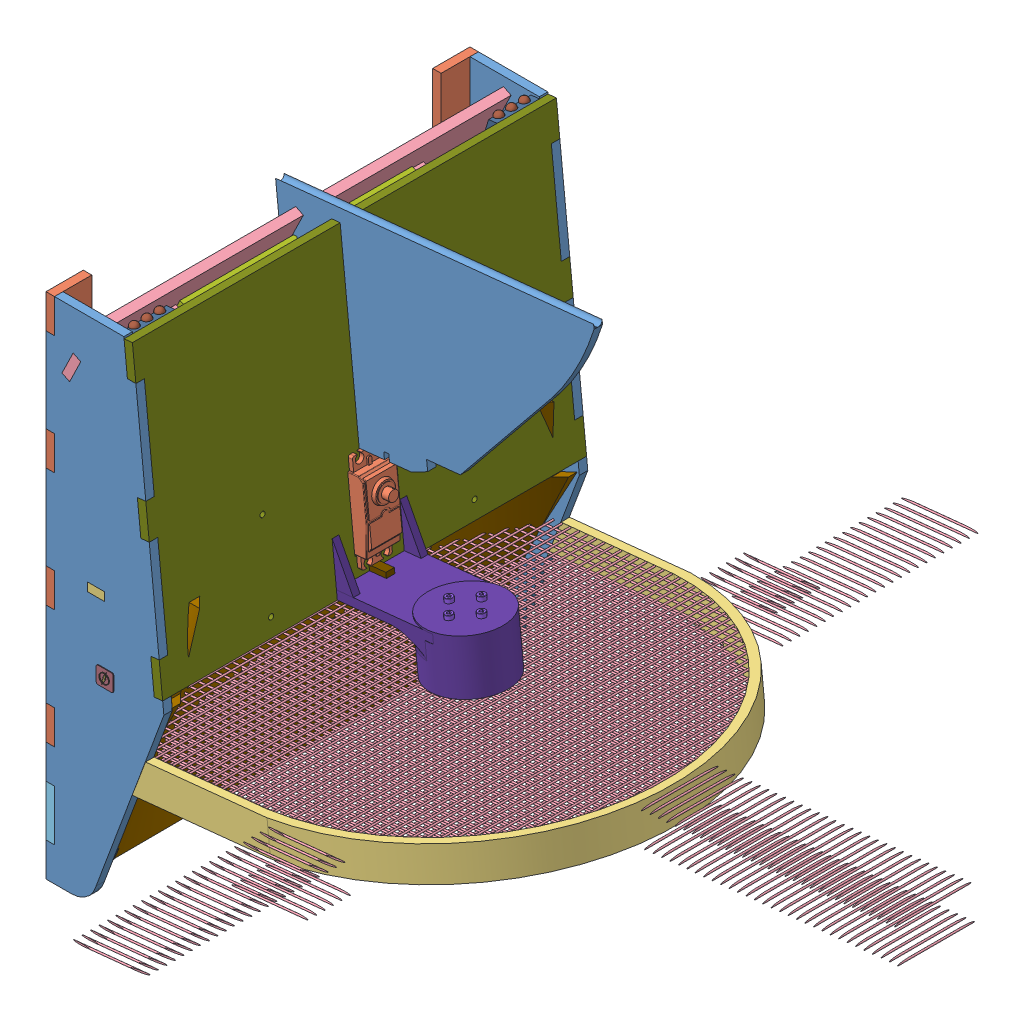
SolidWorks assembly AssStructSimu, configuration Défaut. Lengths in mm. (continued)
Components (placement in the parent): (continued)
- AssCarte-1: AssCarte [Défaut] at (38.0121 147.1029 290.772) x (-0.101852 0.9948 0) z (0.9948 0.101852 0) size (66.52 130.57 98.72) (hidden) (continued)
  - carte_onduleur_v3-1: carte_onduleur_v3 [Défaut] at (-131.8199 12.0892 20.7912) size (66.52 130.57 82.34) (continued)
    - CON_IO1-1: CON_IO1 [Défaut] at (-11.3 12.1 0.803) x (0 -1 0) z (0 0 1) size (13 30 57.5) (continued)
      - Open CASCADE STEP translator 6.8 1.3.1-1: Open CASCADE STEP translator 6.8 1.3.1 [Défaut] at origin size (13 30 57.5) (continued)
        - Body_1_2-1: Body_1_2 [Défaut] at (-3 -15 8) x (0 -1 0) z (-1 0 0) size (30 57.5 13) (continued)
          - 74-1: 74 [Défaut] at (-4.9 41.8 0.803) x (0 -1 0) z (0 0 1) size (6 4.9 1.75) (continued)
            - =_[0_1_1_56]-1: =_[0_1_1_56] [Défaut] at origin size (6 4.9 1.75) (continued)
              - 72-1: 72 [Défaut] at origin size (6 4.9 1.75)
                - =_[0_1_1_2]-1: =_[0_1_1_2] [Défaut] at origin size (3.9 4.9 1.57)
                - =_[0_1_1_3]-1: =_[0_1_1_3] [Défaut] at origin size (6 4.22 1)
                  - =_[0_1_1_60]-1: =_[0_1_1_60] [Défaut] at origin size (1.05 0.41 1)
                  - =_[0_1_1_61]-1: =_[0_1_1_61] [Défaut] at origin size (1.05 0.41 1)
                  - =_[0_1_1_62]-1: =_[0_1_1_62] [Défaut] at origin size (1.05 0.41 1)
                  - =_[0_1_1_63]-1: =_[0_1_1_63] [Défaut] at origin size (1.05 0.41 1)
                  - =_[0_1_1_64]-1: =_[0_1_1_64] [Défaut] at origin size (1.05 0.41 1)
                  - =_[0_1_1_65]-1: =_[0_1_1_65] [Défaut] at origin size (1.05 0.41 1)
                  - =_[0_1_1_66]-1: =_[0_1_1_66] [Défaut] at origin size (1.05 0.41 1)
                  - =_[0_1_1_67]-1: =_[0_1_1_67] [Défaut] at origin size (1.05 0.41 1)
          - 76-1: 76 [Défaut] at (-8.5 40.5664 0.803) x (0 1 0) z (0 0 1) size (2.34 1.04 0.5)
            - =_[0_1_1_42]-1: =_[0_1_1_42] [Défaut] at origin size (2.34 1.04 0.5)
              - 43-1: 43 [Défaut] at origin size (2.29 1.04 0.43)
              - 44-1: 44 [Défaut] at (0.3048 0 0) x (-1 0 0) z (0 0 1) size (0.51 1.02 0.5)
              - 45-1: 45 [Défaut] at origin size (0.51 1.02 0.5)
          - 78-1: 78 [Défaut] at (-5.9 46.4 0.803) x (-1 0 0) z (0 0 1) size (2.34 1.04 0.5)
            - =_[0_1_1_42]-1: =_[0_1_1_42] [Défaut] at origin size (2.34 1.04 0.5)
              - 43-1: 43 [Défaut] at origin size (2.29 1.04 0.43)
              - 44-1: 44 [Défaut] at (0.3048 0 0) x (-1 0 0) z (0 0 1) size (0.51 1.02 0.5)
              - 45-1: 45 [Défaut] at origin size (0.51 1.02 0.5)
          - 80-1: 80 [Défaut] at (-7 48.1 0.803) size (2.34 1.04 0.5)
            - =_[0_1_1_42]-1: =_[0_1_1_42] [Défaut] at origin size (2.34 1.04 0.5)
              - 43-1: 43 [Défaut] at origin size (2.29 1.04 0.43)
              - 44-1: 44 [Défaut] at (0.3048 0 0) x (-1 0 0) z (0 0 1) size (0.51 1.02 0.5)
              - 45-1: 45 [Défaut] at origin size (0.51 1.02 0.5)
          - 82-1: 82 [Défaut] at (-6 37.1 0.803) size (2.34 1.04 0.5)
            - =_[0_1_1_42]-1: =_[0_1_1_42] [Défaut] at origin size (2.34 1.04 0.5)
              - 43-1: 43 [Défaut] at origin size (2.29 1.04 0.43)
              - 44-1: 44 [Défaut] at (0.3048 0 0) x (-1 0 0) z (0 0 1) size (0.51 1.02 0.5)
              - 45-1: 45 [Défaut] at origin size (0.51 1.02 0.5)
    - CON_IO2-1: CON_IO2 [Défaut] at (-11.3 -2.7 0.803) x (0 -1 0) z (0 0 1) size (13 30 57.5)
      - Open CASCADE STEP translator 6.8 1.4.1-1: Open CASCADE STEP translator 6.8 1.4.1 [Défaut] at origin size (13 30 57.5)
        - Body_1_2-1: Body_1_2 [Défaut] at (-3 -15 8) x (0 -1 0) z (-1 0 0) size (30 57.5 13)
          - 1-1: 1 [Défaut] at origin size (30 50 1.61)
          - 10-1: 10 [Défaut] at (-14.395 31.0465 0.803) x (-1 0 0) z (0 0 1) size (5.59 6.35 1.11)
            - =_[0_1_1_4]-1: =_[0_1_1_4] [Défaut] at origin size (5.59 6.35 1.11)
              - 11-1: 11 [Défaut] at (2 3.3 0) x (-1 0 0) z (0 0 1) size (5.59 6.35 1.11)
                - =_[0_1_1_3]_2-1: =_[0_1_1_3]_2 [Défaut] at origin size (0.44 0.55 0.36)
                - =_[0_1_1_4]_2-1: =_[0_1_1_4]_2 [Défaut] at origin size (5.59 4.15 0.36)
                - =_[0_1_1_5]_2-1: =_[0_1_1_5]_2 [Défaut] at origin size (5.35 6.1 1.1)
                - =_[0_1_1_6]-1: =_[0_1_1_6] [Défaut] at origin size (0.44 0.55 0.36)
                - =_[0_1_1_7]-1: =_[0_1_1_7] [Défaut] at origin size (0.44 0.55 0.36)
                - =_[0_1_1_8]-1: =_[0_1_1_8] [Défaut] at origin size (0.44 0.55 0.36)
          - 13-1: 13 [Défaut] at (-12.62 16.6 -0.803) x (-1 0 0) z (0 0 -1) size (5.59 6.35 1.11)
            - =_[0_1_1_13]-1: =_[0_1_1_13] [Défaut] at origin size (5.59 6.35 1.11)
              - 11-1: 11 [Défaut] at (2 3.3 0) x (-1 0 0) z (0 0 1) size (5.59 6.35 1.11)
                - =_[0_1_1_3]_2-1: =_[0_1_1_3]_2 [Défaut] at origin size (0.44 0.55 0.36)
                - =_[0_1_1_4]_2-1: =_[0_1_1_4]_2 [Défaut] at origin size (5.59 4.15 0.36)
                - =_[0_1_1_5]_2-1: =_[0_1_1_5]_2 [Défaut] at origin size (5.35 6.1 1.1)
                - =_[0_1_1_6]-1: =_[0_1_1_6] [Défaut] at origin size (0.44 0.55 0.36)
                - =_[0_1_1_7]-1: =_[0_1_1_7] [Défaut] at origin size (0.44 0.55 0.36)
                - =_[0_1_1_8]-1: =_[0_1_1_8] [Défaut] at origin size (0.44 0.55 0.36)
          - 16-1: 16 [Défaut] at (-4.2 24.2 0.803) x (-1 0 0) z (0 0 1) size (12.8 0.5 13)
            - =_[0_1_1_15]-1: =_[0_1_1_15] [Défaut] at origin size (12.8 0.5 13)
              - 17-1: 17 [Défaut] at (2.7 0 0) x (1 0 0) z (0 -1 0) size (12.8 13 0.5)
          - 19-1: 19 [Défaut] at (-4.1 6.8 0.803) x (-1 0 0) z (0 0 1) size (12.8 0.5 13)
            - =_[0_1_1_18]-1: =_[0_1_1_18] [Défaut] at origin size (12.8 0.5 13)
              - 17-1: 17 [Défaut] at (2.7 0 0) x (1 0 0) z (0 -1 0) size (12.8 13 0.5)
          - 24-1: 24 [Défaut] at (-8.1 16.5 -0.803) x (0 1 0) z (0 0 -1) size (7.75 5.13 1.17)
            - =_[0_1_1_20]-1: =_[0_1_1_20] [Défaut] at origin size (7.75 5.13 1.17)
              - 20-1: 20 [Défaut] at origin size (7.59 5.13 1.07)
              - 21-1: 21 [Défaut] at (-14.478 0 0) x (-1 0 0) z (0 0 1) size (0.76 5.08 1.17)
              - 22-1: 22 [Défaut] at origin size (0.76 5.08 1.17)
          - 35-1: 35 [Défaut] at (-25.3 25.5 0.803) x (0 -1 0) z (0 0 1) size (6.05 5.2 1.7)
            - =_[0_1_1_25]-1: =_[0_1_1_25] [Défaut] at origin size (6.05 5.2 1.7)
              - 25-1: 25 [Défaut] at origin size (4.3 5.2 1.53)
              - 26-1: 26 [Défaut] at origin size (0.88 0.51 1.06)
              - 27-1: 27 [Défaut] at origin size (0.88 0.51 1.06)
              - 28-1: 28 [Défaut] at origin size (0.88 0.51 1.06)
              - 29-1: 29 [Défaut] at origin size (0.88 0.51 1.06)
              - 30-1: 30 [Défaut] at (11.6 -5.08 0) x (-1 0 0) z (0 0 1) size (0.87 0.51 1.06)
              - 31-1: 31 [Défaut] at (11.6 -2.54 0) x (-1 0 0) z (0 0 1) size (0.87 0.51 1.06)
              - 32-1: 32 [Défaut] at (11.6 0 0) x (-1 0 0) z (0 0 1) size (0.87 0.51 1.06)
              - 33-1: 33 [Défaut] at (11.6 2.54 0) x (-1 0 0) z (0 0 1) size (0.87 0.51 1.06)
          - 40-1: 40 [Défaut] at (-27.6 27.2 0.803) size (2.34 1.04 0.5)
            - =_[0_1_1_36]-1: =_[0_1_1_36] [Défaut] at origin size (2.34 1.04 0.5)
              - 36-1: 36 [Défaut] at origin size (2.29 1.04 0.43)
              - 37-1: 37 [Défaut] at (0.3048 0 0) x (-1 0 0) z (0 0 1) size (0.51 1.02 0.5)
              - 38-1: 38 [Défaut] at origin size (0.51 1.02 0.5)
          - 42-1: 42 [Défaut] at (-22.1 21.6 0.803) x (0 1 0) z (0 0 1) size (2.34 1.04 0.5)
            - =_[0_1_1_36]-1: =_[0_1_1_36] [Défaut] at origin size (2.34 1.04 0.5)
              - 36-1: 36 [Défaut] at origin size (2.29 1.04 0.43)
              - 37-1: 37 [Défaut] at (0.3048 0 0) x (-1 0 0) z (0 0 1) size (0.51 1.02 0.5)
              - 38-1: 38 [Défaut] at origin size (0.51 1.02 0.5)
          - 47-1: 47 [Défaut] at (-14.7664 14.5 -0.803) x (-1 0 0) z (0 0 -1) size (2.34 1.04 0.5)
            - =_[0_1_1_42]-1: =_[0_1_1_42] [Défaut] at origin size (2.34 1.04 0.5)
              - 43-1: 43 [Défaut] at origin size (2.29 1.04 0.43)
              - 44-1: 44 [Défaut] at (0.3048 0 0) x (-1 0 0) z (0 0 1) size (0.51 1.02 0.5)
              - 45-1: 45 [Défaut] at origin size (0.51 1.02 0.5)
          - 57-1: 57 [Défaut] at (-15.3 2.7 -0.803) x (0 -1 0) z (0 0 -1) size (10.36 15.24 6.14)
            - =_[0_1_1_47]-1: =_[0_1_1_47] [Défaut] at origin size (10.36 15.24 6.14)
              - 55-1: 55 [Défaut] at (1.8 -1.2 3) x (1 0 0) z (0 1 0) size (10.36 6.14 15.24)
                - 54-1: 54 [Défaut] at origin size (10.36 6.14 7.62)
                  - 52-1: 52 [Défaut] at origin size (10.36 6.14 2.54)
                    - 48-1: 48 [Défaut] at origin size (8.4 2.54 2.54)
                    - 49-1: 49 [Défaut] at (-0.0461 1.2682 1.27) x (0 0 -1) z (0.999998 -0.002105 0) size (1.95 5.07 7.58)
                  - 52-2: 52 [Défaut] at (0 0 -2.54) size (10.36 6.14 2.54)
                    - 48-1: 48 [Défaut] at origin size (8.4 2.54 2.54)
                    - 49-1: 49 [Défaut] at (-0.0461 1.2682 1.27) x (0 0 -1) z (0.999998 -0.002105 0) size (1.95 5.07 7.58)
                  - 52-3: 52 [Défaut] at (0 0 -5.08) size (10.36 6.14 2.54)
                    - 48-1: 48 [Défaut] at origin size (8.4 2.54 2.54)
                    - 49-1: 49 [Défaut] at (-0.0461 1.2682 1.27) x (0 0 -1) z (0.999998 -0.002105 0) size (1.95 5.07 7.58)
                - 54-2: 54 [Défaut] at (0 0 -7.62) size (10.36 6.14 7.62)
                  - 52-1: 52 [Défaut] at origin size (10.36 6.14 2.54)
                    - 48-1: 48 [Défaut] at origin size (8.4 2.54 2.54)
                    - 49-1: 49 [Défaut] at (-0.0461 1.2682 1.27) x (0 0 -1) z (0.999998 -0.002105 0) size (1.95 5.07 7.58)
                  - 52-2: 52 [Défaut] at (0 0 -2.54) size (10.36 6.14 2.54)
                    - 48-1: 48 [Défaut] at origin size (8.4 2.54 2.54)
                    - 49-1: 49 [Défaut] at (-0.0461 1.2682 1.27) x (0 0 -1) z (0.999998 -0.002105 0) size (1.95 5.07 7.58)
                  - 52-3: 52 [Défaut] at (0 0 -5.08) size (10.36 6.14 2.54)
                    - 48-1: 48 [Défaut] at origin size (8.4 2.54 2.54)
                    - 49-1: 49 [Défaut] at (-0.0461 1.2682 1.27) x (0 0 -1) z (0.999998 -0.002105 0) size (1.95 5.07 7.58)
          - 59-1: 59 [Défaut] at (-26.5 31 0.803) x (0 -1 0) z (0 0 1) size (2.34 1.04 0.5)
            - =_[0_1_1_42]-1: =_[0_1_1_42] [Défaut] at origin size (2.34 1.04 0.5)
              - 43-1: 43 [Défaut] at origin size (2.29 1.04 0.43)
              - 44-1: 44 [Défaut] at (0.3048 0 0) x (-1 0 0) z (0 0 1) size (0.51 1.02 0.5)
              - 45-1: 45 [Défaut] at origin size (0.51 1.02 0.5)
          - 61-1: 61 [Défaut] at (-21.6 17.8 0.803) x (-1 0 0) z (0 0 1) size (2.34 1.04 0.5)
            - =_[0_1_1_42]-1: =_[0_1_1_42] [Défaut] at origin size (2.34 1.04 0.5)
              - 43-1: 43 [Défaut] at origin size (2.29 1.04 0.43)
              - 44-1: 44 [Défaut] at (0.3048 0 0) x (-1 0 0) z (0 0 1) size (0.51 1.02 0.5)
              - 45-1: 45 [Défaut] at origin size (0.51 1.02 0.5)
          - 74-1: 74 [Défaut] at (-4.9 41.8 0.803) x (0 -1 0) z (0 0 1) size (6 4.9 1.75)
            - =_[0_1_1_56]-1: =_[0_1_1_56] [Défaut] at origin size (6 4.9 1.75)
              - 72-1: 72 [Défaut] at origin size (6 4.9 1.75)
                - =_[0_1_1_2]-1: =_[0_1_1_2] [Défaut] at origin size (3.9 4.9 1.57)
                - =_[0_1_1_3]-1: =_[0_1_1_3] [Défaut] at origin size (6 4.22 1)
                  - =_[0_1_1_60]-1: =_[0_1_1_60] [Défaut] at origin size (1.05 0.41 1)
                  - =_[0_1_1_61]-1: =_[0_1_1_61] [Défaut] at origin size (1.05 0.41 1)
                  - =_[0_1_1_62]-1: =_[0_1_1_62] [Défaut] at origin size (1.05 0.41 1)
                  - =_[0_1_1_63]-1: =_[0_1_1_63] [Défaut] at origin size (1.05 0.41 1)
                  - =_[0_1_1_64]-1: =_[0_1_1_64] [Défaut] at origin size (1.05 0.41 1)
                  - =_[0_1_1_65]-1: =_[0_1_1_65] [Défaut] at origin size (1.05 0.41 1)
                  - =_[0_1_1_66]-1: =_[0_1_1_66] [Défaut] at origin size (1.05 0.41 1)
                  - =_[0_1_1_67]-1: =_[0_1_1_67] [Défaut] at origin size (1.05 0.41 1)
          - 76-1: 76 [Défaut] at (-8.5 40.5664 0.803) x (0 1 0) z (0 0 1) size (2.34 1.04 0.5)
            - =_[0_1_1_42]-1: =_[0_1_1_42] [Défaut] at origin size (2.34 1.04 0.5)
              - 43-1: 43 [Défaut] at origin size (2.29 1.04 0.43)
              - 44-1: 44 [Défaut] at (0.3048 0 0) x (-1 0 0) z (0 0 1) size (0.51 1.02 0.5)
              - 45-1: 45 [Défaut] at origin size (0.51 1.02 0.5)
          - 78-1: 78 [Défaut] at (-5.9 46.4 0.803) x (-1 0 0) z (0 0 1) size (2.34 1.04 0.5)
            - =_[0_1_1_42]-1: =_[0_1_1_42] [Défaut] at origin size (2.34 1.04 0.5)
              - 43-1: 43 [Défaut] at origin size (2.29 1.04 0.43)
              - 44-1: 44 [Défaut] at (0.3048 0 0) x (-1 0 0) z (0 0 1) size (0.51 1.02 0.5)
              - 45-1: 45 [Défaut] at origin size (0.51 1.02 0.5)
          - 80-1: 80 [Défaut] at (-7 48.1 0.803) size (2.34 1.04 0.5)
            - =_[0_1_1_42]-1: =_[0_1_1_42] [Défaut] at origin size (2.34 1.04 0.5)
              - 43-1: 43 [Défaut] at origin size (2.29 1.04 0.43)
              - 44-1: 44 [Défaut] at (0.3048 0 0) x (-1 0 0) z (0 0 1) size (0.51 1.02 0.5)
              - 45-1: 45 [Défaut] at origin size (0.51 1.02 0.5)
          - 82-1: 82 [Défaut] at (-6 37.1 0.803) size (2.34 1.04 0.5)
            - =_[0_1_1_42]-1: =_[0_1_1_42] [Défaut] at origin size (2.34 1.04 0.5)
              - 43-1: 43 [Défaut] at origin size (2.29 1.04 0.43)
              - 44-1: 44 [Défaut] at (0.3048 0 0) x (-1 0 0) z (0 0 1) size (0.51 1.02 0.5)
              - 45-1: 45 [Défaut] at origin size (0.51 1.02 0.5)
    - CON_IO3-1: CON_IO3 [Défaut] at (-11.3 -17.7 0.803) x (0 -1 0) z (0 0 1) size (13 30 57.5)
      - Open CASCADE STEP translator 6.8 1.5.1-1: Open CASCADE STEP translator 6.8 1.5.1 [Défaut] at origin size (13 30 57.5)
        - Body_1_2-1: Body_1_2 [Défaut] at (-3 -15 8) x (0 -1 0) z (-1 0 0) size (30 57.5 13)
          - 1-1: 1 [Défaut] at origin size (30 50 1.61)
          - 10-1: 10 [Défaut] at (-14.395 31.0465 0.803) x (-1 0 0) z (0 0 1) size (5.59 6.35 1.11)
            - =_[0_1_1_4]-1: =_[0_1_1_4] [Défaut] at origin size (5.59 6.35 1.11)
              - 11-1: 11 [Défaut] at (2 3.3 0) x (-1 0 0) z (0 0 1) size (5.59 6.35 1.11)
                - =_[0_1_1_3]_2-1: =_[0_1_1_3]_2 [Défaut] at origin size (0.44 0.55 0.36)
                - =_[0_1_1_4]_2-1: =_[0_1_1_4]_2 [Défaut] at origin size (5.59 4.15 0.36)
                - =_[0_1_1_5]_2-1: =_[0_1_1_5]_2 [Défaut] at origin size (5.35 6.1 1.1)
                - =_[0_1_1_6]-1: =_[0_1_1_6] [Défaut] at origin size (0.44 0.55 0.36)
                - =_[0_1_1_7]-1: =_[0_1_1_7] [Défaut] at origin size (0.44 0.55 0.36)
                - =_[0_1_1_8]-1: =_[0_1_1_8] [Défaut] at origin size (0.44 0.55 0.36)
          - 13-1: 13 [Défaut] at (-12.62 16.6 -0.803) x (-1 0 0) z (0 0 -1) size (5.59 6.35 1.11)
            - =_[0_1_1_13]-1: =_[0_1_1_13] [Défaut] at origin size (5.59 6.35 1.11)
              - 11-1: 11 [Défaut] at (2 3.3 0) x (-1 0 0) z (0 0 1) size (5.59 6.35 1.11)
                - =_[0_1_1_3]_2-1: =_[0_1_1_3]_2 [Défaut] at origin size (0.44 0.55 0.36)
                - =_[0_1_1_4]_2-1: =_[0_1_1_4]_2 [Défaut] at origin size (5.59 4.15 0.36)
                - =_[0_1_1_5]_2-1: =_[0_1_1_5]_2 [Défaut] at origin size (5.35 6.1 1.1)
                - =_[0_1_1_6]-1: =_[0_1_1_6] [Défaut] at origin size (0.44 0.55 0.36)
                - =_[0_1_1_7]-1: =_[0_1_1_7] [Défaut] at origin size (0.44 0.55 0.36)
                - =_[0_1_1_8]-1: =_[0_1_1_8] [Défaut] at origin size (0.44 0.55 0.36)
          - 16-1: 16 [Défaut] at (-4.2 24.2 0.803) x (-1 0 0) z (0 0 1) size (12.8 0.5 13)
            - =_[0_1_1_15]-1: =_[0_1_1_15] [Défaut] at origin size (12.8 0.5 13)
              - 17-1: 17 [Défaut] at (2.7 0 0) x (1 0 0) z (0 -1 0) size (12.8 13 0.5)
          - 19-1: 19 [Défaut] at (-4.1 6.8 0.803) x (-1 0 0) z (0 0 1) size (12.8 0.5 13)
            - =_[0_1_1_18]-1: =_[0_1_1_18] [Défaut] at origin size (12.8 0.5 13)
              - 17-1: 17 [Défaut] at (2.7 0 0) x (1 0 0) z (0 -1 0) size (12.8 13 0.5)
          - 24-1: 24 [Défaut] at (-8.1 16.5 -0.803) x (0 1 0) z (0 0 -1) size (7.75 5.13 1.17)
            - =_[0_1_1_20]-1: =_[0_1_1_20] [Défaut] at origin size (7.75 5.13 1.17)
              - 20-1: 20 [Défaut] at origin size (7.59 5.13 1.07)
              - 21-1: 21 [Défaut] at (-14.478 0 0) x (-1 0 0) z (0 0 1) size (0.76 5.08 1.17)
              - 22-1: 22 [Défaut] at origin size (0.76 5.08 1.17)
          - 35-1: 35 [Défaut] at (-25.3 25.5 0.803) x (0 -1 0) z (0 0 1) size (6.05 5.2 1.7)
            - =_[0_1_1_25]-1: =_[0_1_1_25] [Défaut] at origin size (6.05 5.2 1.7)
              - 25-1: 25 [Défaut] at origin size (4.3 5.2 1.53)
              - 26-1: 26 [Défaut] at origin size (0.88 0.51 1.06)
              - 27-1: 27 [Défaut] at origin size (0.88 0.51 1.06)
              - 28-1: 28 [Défaut] at origin size (0.88 0.51 1.06)
              - 29-1: 29 [Défaut] at origin size (0.88 0.51 1.06)
              - 30-1: 30 [Défaut] at (11.6 -5.08 0) x (-1 0 0) z (0 0 1) size (0.87 0.51 1.06)
              - 31-1: 31 [Défaut] at (11.6 -2.54 0) x (-1 0 0) z (0 0 1) size (0.87 0.51 1.06)
              - 32-1: 32 [Défaut] at (11.6 0 0) x (-1 0 0) z (0 0 1) size (0.87 0.51 1.06)
              - 33-1: 33 [Défaut] at (11.6 2.54 0) x (-1 0 0) z (0 0 1) size (0.87 0.51 1.06)
          - 40-1: 40 [Défaut] at (-27.6 27.2 0.803) size (2.34 1.04 0.5)
            - =_[0_1_1_36]-1: =_[0_1_1_36] [Défaut] at origin size (2.34 1.04 0.5)
              - 36-1: 36 [Défaut] at origin size (2.29 1.04 0.43)
              - 37-1: 37 [Défaut] at (0.3048 0 0) x (-1 0 0) z (0 0 1) size (0.51 1.02 0.5)
              - 38-1: 38 [Défaut] at origin size (0.51 1.02 0.5)
          - 42-1: 42 [Défaut] at (-22.1 21.6 0.803) x (0 1 0) z (0 0 1) size (2.34 1.04 0.5)
            - =_[0_1_1_36]-1: =_[0_1_1_36] [Défaut] at origin size (2.34 1.04 0.5)
              - 36-1: 36 [Défaut] at origin size (2.29 1.04 0.43)
              - 37-1: 37 [Défaut] at (0.3048 0 0) x (-1 0 0) z (0 0 1) size (0.51 1.02 0.5)
              - 38-1: 38 [Défaut] at origin size (0.51 1.02 0.5)
          - 47-1: 47 [Défaut] at (-14.7664 14.5 -0.803) x (-1 0 0) z (0 0 -1) size (2.34 1.04 0.5)
            - =_[0_1_1_42]-1: =_[0_1_1_42] [Défaut] at origin size (2.34 1.04 0.5)
              - 43-1: 43 [Défaut] at origin size (2.29 1.04 0.43)
              - 44-1: 44 [Défaut] at (0.3048 0 0) x (-1 0 0) z (0 0 1) size (0.51 1.02 0.5)
              - 45-1: 45 [Défaut] at origin size (0.51 1.02 0.5)
          - 57-1: 57 [Défaut] at (-15.3 2.7 -0.803) x (0 -1 0) z (0 0 -1) size (10.36 15.24 6.14)
            - =_[0_1_1_47]-1: =_[0_1_1_47] [Défaut] at origin size (10.36 15.24 6.14)
              - 55-1: 55 [Défaut] at (1.8 -1.2 3) x (1 0 0) z (0 1 0) size (10.36 6.14 15.24)
                - 54-1: 54 [Défaut] at origin size (10.36 6.14 7.62)
                  - 52-1: 52 [Défaut] at origin size (10.36 6.14 2.54)
                    - 48-1: 48 [Défaut] at origin size (8.4 2.54 2.54)
                    - 49-1: 49 [Défaut] at (-0.0461 1.2682 1.27) x (0 0 -1) z (0.999998 -0.002105 0) size (1.95 5.07 7.58)
                  - 52-2: 52 [Défaut] at (0 0 -2.54) size (10.36 6.14 2.54)
                    - 48-1: 48 [Défaut] at origin size (8.4 2.54 2.54)
                    - 49-1: 49 [Défaut] at (-0.0461 1.2682 1.27) x (0 0 -1) z (0.999998 -0.002105 0) size (1.95 5.07 7.58)
                  - 52-3: 52 [Défaut] at (0 0 -5.08) size (10.36 6.14 2.54)
                    - 48-1: 48 [Défaut] at origin size (8.4 2.54 2.54)
                    - 49-1: 49 [Défaut] at (-0.0461 1.2682 1.27) x (0 0 -1) z (0.999998 -0.002105 0) size (1.95 5.07 7.58)
                - 54-2: 54 [Défaut] at (0 0 -7.62) size (10.36 6.14 7.62)
                  - 52-1: 52 [Défaut] at origin size (10.36 6.14 2.54)
                    - 48-1: 48 [Défaut] at origin size (8.4 2.54 2.54)
                    - 49-1: 49 [Défaut] at (-0.0461 1.2682 1.27) x (0 0 -1) z (0.999998 -0.002105 0) size (1.95 5.07 7.58)
                  - 52-2: 52 [Défaut] at (0 0 -2.54) size (10.36 6.14 2.54)
                    - 48-1: 48 [Défaut] at origin size (8.4 2.54 2.54)
                    - 49-1: 49 [Défaut] at (-0.0461 1.2682 1.27) x (0 0 -1) z (0.999998 -0.002105 0) size (1.95 5.07 7.58)
                  - 52-3: 52 [Défaut] at (0 0 -5.08) size (10.36 6.14 2.54)
                    - 48-1: 48 [Défaut] at origin size (8.4 2.54 2.54)
                    - 49-1: 49 [Défaut] at (-0.0461 1.2682 1.27) x (0 0 -1) z (0.999998 -0.002105 0) size (1.95 5.07 7.58)
          - 59-1: 59 [Défaut] at (-26.5 31 0.803) x (0 -1 0) z (0 0 1) size (2.34 1.04 0.5)
            - =_[0_1_1_42]-1: =_[0_1_1_42] [Défaut] at origin size (2.34 1.04 0.5)
              - 43-1: 43 [Défaut] at origin size (2.29 1.04 0.43)
              - 44-1: 44 [Défaut] at (0.3048 0 0) x (-1 0 0) z (0 0 1) size (0.51 1.02 0.5)
              - 45-1: 45 [Défaut] at origin size (0.51 1.02 0.5)
          - 61-1: 61 [Défaut] at (-21.6 17.8 0.803) x (-1 0 0) z (0 0 1) size (2.34 1.04 0.5)
            - =_[0_1_1_42]-1: =_[0_1_1_42] [Défaut] at origin size (2.34 1.04 0.5)
              - 43-1: 43 [Défaut] at origin size (2.29 1.04 0.43)
              - 44-1: 44 [Défaut] at (0.3048 0 0) x (-1 0 0) z (0 0 1) size (0.51 1.02 0.5)
              - 45-1: 45 [Défaut] at origin size (0.51 1.02 0.5)
          - 74-1: 74 [Défaut] at (-4.9 41.8 0.803) x (0 -1 0) z (0 0 1) size (6 4.9 1.75)
            - =_[0_1_1_56]-1: =_[0_1_1_56] [Défaut] at origin size (6 4.9 1.75)
              - 72-1: 72 [Défaut] at origin size (6 4.9 1.75)
                - =_[0_1_1_2]-1: =_[0_1_1_2] [Défaut] at origin size (3.9 4.9 1.57)
                - =_[0_1_1_3]-1: =_[0_1_1_3] [Défaut] at origin size (6 4.22 1)
                  - =_[0_1_1_60]-1: =_[0_1_1_60] [Défaut] at origin size (1.05 0.41 1)
                  - =_[0_1_1_61]-1: =_[0_1_1_61] [Défaut] at origin size (1.05 0.41 1)
                  - =_[0_1_1_62]-1: =_[0_1_1_62] [Défaut] at origin size (1.05 0.41 1)
                  - =_[0_1_1_63]-1: =_[0_1_1_63] [Défaut] at origin size (1.05 0.41 1)
                  - =_[0_1_1_64]-1: =_[0_1_1_64] [Défaut] at origin size (1.05 0.41 1)
                  - =_[0_1_1_65]-1: =_[0_1_1_65] [Défaut] at origin size (1.05 0.41 1)
                  - =_[0_1_1_66]-1: =_[0_1_1_66] [Défaut] at origin size (1.05 0.41 1)
                  - =_[0_1_1_67]-1: =_[0_1_1_67] [Défaut] at origin size (1.05 0.41 1)
          - 76-1: 76 [Défaut] at (-8.5 40.5664 0.803) x (0 1 0) z (0 0 1) size (2.34 1.04 0.5)
            - =_[0_1_1_42]-1: =_[0_1_1_42] [Défaut] at origin size (2.34 1.04 0.5)
              - 43-1: 43 [Défaut] at origin size (2.29 1.04 0.43)
              - 44-1: 44 [Défaut] at (0.3048 0 0) x (-1 0 0) z (0 0 1) size (0.51 1.02 0.5)
              - 45-1: 45 [Défaut] at origin size (0.51 1.02 0.5)
          - 78-1: 78 [Défaut] at (-5.9 46.4 0.803) x (-1 0 0) z (0 0 1) size (2.34 1.04 0.5)
            - =_[0_1_1_42]-1: =_[0_1_1_42] [Défaut] at origin size (2.34 1.04 0.5)
              - 43-1: 43 [Défaut] at origin size (2.29 1.04 0.43)
              - 44-1: 44 [Défaut] at (0.3048 0 0) x (-1 0 0) z (0 0 1) size (0.51 1.02 0.5)
              - 45-1: 45 [Défaut] at origin size (0.51 1.02 0.5)
          - 80-1: 80 [Défaut] at (-7 48.1 0.803) size (2.34 1.04 0.5)
            - =_[0_1_1_42]-1: =_[0_1_1_42] [Défaut] at origin size (2.34 1.04 0.5)
              - 43-1: 43 [Défaut] at origin size (2.29 1.04 0.43)
              - 44-1: 44 [Défaut] at (0.3048 0 0) x (-1 0 0) z (0 0 1) size (0.51 1.02 0.5)
              - 45-1: 45 [Défaut] at origin size (0.51 1.02 0.5)
          - 82-1: 82 [Défaut] at (-6 37.1 0.803) size (2.34 1.04 0.5)
            - =_[0_1_1_42]-1: =_[0_1_1_42] [Défaut] at origin size (2.34 1.04 0.5)
              - 43-1: 43 [Défaut] at origin size (2.29 1.04 0.43)
              - 44-1: 44 [Défaut] at (0.3048 0 0) x (-1 0 0) z (0 0 1) size (0.51 1.02 0.5)
              - 45-1: 45 [Défaut] at origin size (0.51 1.02 0.5)
    - C1_1-1: C1_1 [Défaut] at (-20.6336 6.4 -0.803) x (1 0 0) z (0 0 -1) size (2.34 1.04 0.5)
      - Open CASCADE STEP translator 6.8 1.6.1-1: Open CASCADE STEP translator 6.8 1.6.1 [Défaut] at origin size (2.34 1.04 0.5)
        - Body_1-1: Body_1 [Défaut] at origin size (2.29 1.04 0.43)
        - Pin_1-1: Pin_1 [Défaut] at (0.3048 0 0) x (-1 0 0) z (0 0 1) size (0.51 1.02 0.5)
        - Pin_2-1: Pin_2 [Défaut] at origin size (0.51 1.02 0.5)
    - C1_2-1: C1_2 [Défaut] at (-24.2 6.4 -0.803) x (1 0 0) z (0 0 -1) size (2.34 1.04 0.5)
      - Open CASCADE STEP translator 6.8 1.6.1-1: Open CASCADE STEP translator 6.8 1.6.1 [Défaut] at origin size (2.34 1.04 0.5)
        - Body_1-1: Body_1 [Défaut] at origin size (2.29 1.04 0.43)
        - Pin_1-1: Pin_1 [Défaut] at (0.3048 0 0) x (-1 0 0) z (0 0 1) size (0.51 1.02 0.5)
        - Pin_2-1: Pin_2 [Défaut] at origin size (0.51 1.02 0.5)
    - C_F-1: C_F [Défaut] at (-16.2432 4.45 -0.803) x (0 -1 0) z (0 0 -1) size (2.34 1.04 0.5)
      - Open CASCADE STEP translator 6.8 1.6.1-1: Open CASCADE STEP translator 6.8 1.6.1 [Défaut] at origin size (2.34 1.04 0.5)
        - Body_1-1: Body_1 [Défaut] at origin size (2.29 1.04 0.43)
        - Pin_1-1: Pin_1 [Défaut] at (0.3048 0 0) x (-1 0 0) z (0 0 1) size (0.51 1.02 0.5)
        - Pin_2-1: Pin_2 [Défaut] at origin size (0.51 1.02 0.5)
    - D_LED_STATE1-1: D_LED_STATE1 [Défaut] at (-6.8906 -21.6 0.803) size (2.34 1.04 0.5)
      - Open CASCADE STEP translator 6.8 1.6.1-1: Open CASCADE STEP translator 6.8 1.6.1 [Défaut] at origin size (2.34 1.04 0.5)
        - Body_1-1: Body_1 [Défaut] at origin size (2.29 1.04 0.43)
        - Pin_1-1: Pin_1 [Défaut] at (0.3048 0 0) x (-1 0 0) z (0 0 1) size (0.51 1.02 0.5)
        - Pin_2-1: Pin_2 [Défaut] at origin size (0.51 1.02 0.5)
    - PICKIT-1: PICKIT [Défaut] at (-24.1 -30.5 0.803) size (15.24 5 14.3)
      - Open CASCADE STEP translator 6.8 1.10.1-1: Open CASCADE STEP translator 6.8 1.10.1 [Défaut] at origin size (15.24 5 14.3)
        - Body_1_2-1: Body_1_2 [Défaut] at (6.3 0 12) size (15.24 5 14.3)
    - C_DEC_CUR-1: C_DEC_CUR [Défaut] at (-8.9496 5.7572 -0.803) x (0 1 0) z (0 0 -1) size (2.34 1.04 0.5)
      - Open CASCADE STEP translator 6.8 1.6.1-1: Open CASCADE STEP translator 6.8 1.6.1 [Défaut] at origin size (2.34 1.04 0.5)
        - Body_1-1: Body_1 [Défaut] at origin size (2.29 1.04 0.43)
        - Pin_1-1: Pin_1 [Défaut] at (0.3048 0 0) x (-1 0 0) z (0 0 1) size (0.51 1.02 0.5)
        - Pin_2-1: Pin_2 [Défaut] at origin size (0.51 1.02 0.5)
    - R_F-1: R_F [Défaut] at (-14.65 4.4432 -0.803) x (0 -1 0) z (0 0 -1) size (2.34 1.04 0.5)
      - Open CASCADE STEP translator 6.8 1.12.1-1: Open CASCADE STEP translator 6.8 1.12.1 [Défaut] at origin size (2.34 1.04 0.5)
        - Body_1_3-1: Body_1_3 [Défaut] at origin size (2.29 1.04 0.43)
        - Pin_1_2-1: Pin_1_2 [Défaut] at (0.3048 0 0) x (-1 0 0) z (0 0 1) size (0.51 1.02 0.5)
        - Pin_2_2-1: Pin_2_2 [Défaut] at origin size (0.51 1.02 0.5)
    - R_GAIN1-1: R_GAIN1 [Défaut] at (-13.95 5.7568 -0.803) x (0 1 0) z (0 0 -1) size (2.34 1.04 0.5)
      - Open CASCADE STEP translator 6.8 1.12.1-1: Open CASCADE STEP translator 6.8 1.12.1 [Défaut] at origin size (2.34 1.04 0.5)
        - Body_1_3-1: Body_1_3 [Défaut] at origin size (2.29 1.04 0.43)
        - Pin_1_2-1: Pin_1_2 [Défaut] at (0.3048 0 0) x (-1 0 0) z (0 0 1) size (0.51 1.02 0.5)
        - Pin_2_2-1: Pin_2_2 [Défaut] at origin size (0.51 1.02 0.5)
    - R_GAIN2-1: R_GAIN2 [Défaut] at (-15.65 7.9176 -0.803) x (0 -1 0) z (0 0 -1) size (2.34 1.04 0.5)
      - Open CASCADE STEP translator 6.8 1.12.1-1: Open CASCADE STEP translator 6.8 1.12.1 [Défaut] at origin size (2.34 1.04 0.5)
        - Body_1_3-1: Body_1_3 [Défaut] at origin size (2.29 1.04 0.43)
        - Pin_1_2-1: Pin_1_2 [Défaut] at (0.3048 0 0) x (-1 0 0) z (0 0 1) size (0.51 1.02 0.5)
        - Pin_2_2-1: Pin_2_2 [Défaut] at origin size (0.51 1.02 0.5)
    - R_LED_STATE1-1: R_LED_STATE1 [Défaut] at (-6.9242 -19.9 0.803) size (2.34 1.04 0.5)
      - Open CASCADE STEP translator 6.8 1.12.1-1: Open CASCADE STEP translator 6.8 1.12.1 [Défaut] at origin size (2.34 1.04 0.5)
        - Body_1_3-1: Body_1_3 [Défaut] at origin size (2.29 1.04 0.43)
        - Pin_1_2-1: Pin_1_2 [Défaut] at (0.3048 0 0) x (-1 0 0) z (0 0 1) size (0.51 1.02 0.5)
        - Pin_2_2-1: Pin_2_2 [Défaut] at origin size (0.51 1.02 0.5)
    - R_RESET1-1: R_RESET1 [Défaut] at (-23 7.9 0.803) size (2.34 1.04 0.5)
      - Open CASCADE STEP translator 6.8 1.12.1-1: Open CASCADE STEP translator 6.8 1.12.1 [Défaut] at origin size (2.34 1.04 0.5)
        - Body_1_3-1: Body_1_3 [Défaut] at origin size (2.29 1.04 0.43)
        - Pin_1_2-1: Pin_1_2 [Défaut] at (0.3048 0 0) x (-1 0 0) z (0 0 1) size (0.51 1.02 0.5)
        - Pin_2_2-1: Pin_2_2 [Défaut] at origin size (0.51 1.02 0.5)
    - U_DSPIC-1: U_DSPIC [Défaut] at (1.863 -2.61 0.803) size (7.92 35.56 7.75)
      - Open CASCADE STEP translator 6.8 1.17.1-1: Open CASCADE STEP translator 6.8 1.17.1 [Défaut] at origin size (7.92 35.56 7.75)
        - Body_1_4-1: Body_1_4 [Défaut] at (0 -0.2 4) x (1 0 0) z (0 -1 0) size (7.92 7.75 35.56)
    - C_DEC_DSPIC-1: C_DEC_DSPIC [Défaut] at (7.7 -8.8 -0.803) x (0 1 0) z (0 0 -1) size (2.34 1.04 0.5)
      - Open CASCADE STEP translator 6.8 1.6.1-1: Open CASCADE STEP translator 6.8 1.6.1 [Défaut] at origin size (2.34 1.04 0.5)
        - Body_1-1: Body_1 [Défaut] at origin size (2.29 1.04 0.43)
        - Pin_1-1: Pin_1 [Défaut] at (0.3048 0 0) x (-1 0 0) z (0 0 1) size (0.51 1.02 0.5)
        - Pin_2-1: Pin_2 [Défaut] at origin size (0.51 1.02 0.5)
    - IN-1: IN [Défaut] at (24.3 -5.3 0.803) x (0 1 0) z (0 0 1) size (10.21 15.56 26.9)
      - Open CASCADE STEP translator 6.8 1.19.1-1: Open CASCADE STEP translator 6.8 1.19.1 [Défaut] at origin size (10.21 15.56 26.9)
        - Body_1_3-1: Body_1_3 [Défaut] at (-13.5 1.8 3) x (0 1 0) z (1 0 0) size (15.56 26.9 10.21)
          - Imported-1: Imported [Défaut] at (2.0451 -4.5908 20.9802) size (8.6 15.9 10.16)
          - Imported-2: Imported [Défaut] at (-1.6683 9.1092 15.9802) x (0 0 1) z (-1 0 0) size (10.1 18.2 15.1)
            - Imported_2-1: Imported_2 [Défaut] at origin size (10.1 18.2 15.1)
            - Imported_3-1: Imported_3 [Défaut] at origin size (3.43 12.4 4.99)
            - Imported_4-1: Imported_4 [Défaut] at origin size (3.43 12.4 4.99)
            - Imported_5-1: Imported_5 [Défaut] at origin size (3.9 4.9 7)
            - Imported_6-1: Imported_6 [Défaut] at origin size (3.9 4.9 7)
            - Imported_7-1: Imported_7 [Défaut] at origin size (3.8 3.8 6.92)
            - Imported_8-1: Imported_8 [Défaut] at origin size (3.8 3.8 6.92)
            - Imported_9-1: Imported_9 [Défaut] at origin size (9 2.4 14.2)
    - CARTE_CMD-1: CARTE_CMD [Défaut] at (25 57.2 0.803) size (60.1 130 26.71)
      - Open CASCADE STEP translator 6.8 1.20.1-1: Open CASCADE STEP translator 6.8 1.20.1 [Défaut] at origin size (60.1 130 26.71)
        - Body_1_4-1: Body_1_4 [Défaut] at (-55 5 12) size (60.1 130 26.71)
          - 1_2-1: 1_2 [Défaut] at origin size (60.1 130 1.61)
          - 4-1: 4 [Défaut] at (23.6 -124.9 0.803) x (0 1 0) z (0 0 1) size (5 15.24 14.3)
            - =_[0_1_1_4]_2-1: =_[0_1_1_4]_2 [Défaut] at origin size (5 15.24 14.3)
              - 5-1: 5 [Défaut] at (0 -6.5 -13) x (0 1 0) z (0 0 -1) size (15.24 5 14.3)
          - 7-1: 7 [Défaut] at (23.6 -5 0.803) x (0 1 0) z (0 0 1) size (5 15.24 14.3)
            - =_[0_1_1_7]-1: =_[0_1_1_7] [Défaut] at origin size (5 15.24 14.3)
              - 5-1: 5 [Défaut] at (0 -6.5 -13) x (0 1 0) z (0 0 -1) size (15.24 5 14.3)
          - 10_2-1: 10_2 [Défaut] at (18.4 -115.6 0.803) size (25.4 7.92 7.75)
            - =_[0_1_1_9]-1: =_[0_1_1_9] [Défaut] at origin size (25.4 7.92 7.75)
              - 8-1: 8 [Défaut] at (11.2 4 0) x (0 1 0) z (1 0 0) size (7.92 7.75 25.4)
          - 13_2-1: 13_2 [Défaut] at (55.4 -114.7 0.803) x (-1 0 0) z (0 0 1) size (5 7.62 14.3)
            - =_[0_1_1_12]-1: =_[0_1_1_12] [Défaut] at origin size (5 7.62 14.3)
              - 11-1: 11 [Défaut] at (0 -2.5 11) x (0 -1 0) z (0 0 1) size (7.62 5 14.3)
          - 25-1: 25 [Défaut] at (56.9 -12.8 0.803) x (-1 0 0) z (0 0 1) size (16.02 47.26 11.05)
            - =_[0_1_1_15]_2-1: =_[0_1_1_15]_2 [Défaut] at origin size (16.02 47.26 11.05)
              - 23-1: 23 [Défaut] at (-36.5 21 4) x (0 -1 0) z (1 0 0) size (47.26 11.05 16.02)
                - 14-1: 14 [Défaut] at (-7.4961 -1.5352 42.5833) size (42.58 6.55 16.01)
                - 22-1: 22 [Défaut] at (19.3039 2.3748 37.905) x (-1 0 0) z (0 0 -1) size (10.36 6.14 15.24)
                  - 21-1: 21 [Défaut] at origin size (10.36 6.14 7.62)
                    - 19_2-1: 19_2 [Défaut] at origin size (10.36 6.14 2.54)
                      - 15-1: 15 [Défaut] at origin size (8.4 2.54 2.54)
                      - 16-1: 16 [Défaut] at (-0.0461 1.2682 1.27) x (0 0 -1) z (0.999998 -0.002105 0) size (1.95 5.07 7.58)
                    - 19_2-2: 19_2 [Défaut] at (0 0 -2.54) size (10.36 6.14 2.54)
                      - 15-1: 15 [Défaut] at origin size (8.4 2.54 2.54)
                      - 16-1: 16 [Défaut] at (-0.0461 1.2682 1.27) x (0 0 -1) z (0.999998 -0.002105 0) size (1.95 5.07 7.58)
                    - 19_2-3: 19_2 [Défaut] at (0 0 -5.08) size (10.36 6.14 2.54)
                      - 15-1: 15 [Défaut] at origin size (8.4 2.54 2.54)
                      - 16-1: 16 [Défaut] at (-0.0461 1.2682 1.27) x (0 0 -1) z (0.999998 -0.002105 0) size (1.95 5.07 7.58)
                  - 21-2: 21 [Défaut] at (0 0 -7.62) size (10.36 6.14 7.62)
                    - 19_2-1: 19_2 [Défaut] at origin size (10.36 6.14 2.54)
                      - 15-1: 15 [Défaut] at origin size (8.4 2.54 2.54)
                      - 16-1: 16 [Défaut] at (-0.0461 1.2682 1.27) x (0 0 -1) z (0.999998 -0.002105 0) size (1.95 5.07 7.58)
                    - 19_2-2: 19_2 [Défaut] at (0 0 -2.54) size (10.36 6.14 2.54)
                      - 15-1: 15 [Défaut] at origin size (8.4 2.54 2.54)
                      - 16-1: 16 [Défaut] at (-0.0461 1.2682 1.27) x (0 0 -1) z (0.999998 -0.002105 0) size (1.95 5.07 7.58)
                    - 19_2-3: 19_2 [Défaut] at (0 0 -5.08) size (10.36 6.14 2.54)
                      - 15-1: 15 [Défaut] at origin size (8.4 2.54 2.54)
                      - 16-1: 16 [Défaut] at (-0.0461 1.2682 1.27) x (0 0 -1) z (0.999998 -0.002105 0) size (1.95 5.07 7.58)
          - 31-1: 31 [Défaut] at (12.9 -104.5 0.803) size (6.76 3.64 4.37)
            - =_[0_1_1_24]-1: =_[0_1_1_24] [Défaut] at origin size (6.76 3.64 4.37)
              - 29-1: 29 [Défaut] at (-0.3 -2 0) size (6.76 3.64 4.37)
                - =_[0_1_1_3]_3-1: =_[0_1_1_3]_3 [Défaut] at origin size (6 3.64 4.37)
                - =_[0_1_1_4]_3-1: =_[0_1_1_4]_3 [Défaut] at origin size (0.38 1 0.67)
                - =_[0_1_1_5]_3-1: =_[0_1_1_5]_3 [Défaut] at origin size (0.38 1 0.67)
          - 36-1: 36 [Défaut] at (28.6 -12.2 0.803) x (0 -1 0) z (0 0 1) size (2.34 1.04 0.5)
            - =_[0_1_1_30]-1: =_[0_1_1_30] [Défaut] at origin size (2.34 1.04 0.5)
              - 32_2-1: 32_2 [Défaut] at origin size (2.29 1.04 0.43)
              - 33_2-1: 33_2 [Défaut] at (0.3048 0 0) x (-1 0 0) z (0 0 1) size (0.51 1.02 0.5)
              - 34-1: 34 [Défaut] at origin size (0.51 1.02 0.5)
          - 38-1: 38 [Défaut] at (23.7 -12.2 0.803) x (0 -1 0) z (0 0 1) size (2.34 1.04 0.5)
            - =_[0_1_1_30]-1: =_[0_1_1_30] [Défaut] at origin size (2.34 1.04 0.5)
              - 32_2-1: 32_2 [Défaut] at origin size (2.29 1.04 0.43)
              - 33_2-1: 33_2 [Défaut] at (0.3048 0 0) x (-1 0 0) z (0 0 1) size (0.51 1.02 0.5)
              - 34-1: 34 [Défaut] at origin size (0.51 1.02 0.5)
          - 40_2-1: 40_2 [Défaut] at (26.2 -12.2 0.803) x (0 -1 0) z (0 0 1) size (2.34 1.04 0.5)
            - =_[0_1_1_30]-1: =_[0_1_1_30] [Défaut] at origin size (2.34 1.04 0.5)
              - 32_2-1: 32_2 [Défaut] at origin size (2.29 1.04 0.43)
              - 33_2-1: 33_2 [Défaut] at (0.3048 0 0) x (-1 0 0) z (0 0 1) size (0.51 1.02 0.5)
              - 34-1: 34 [Défaut] at origin size (0.51 1.02 0.5)
          - 42_2-1: 42_2 [Défaut] at (24.4 -119.2 0.803) size (2.34 1.04 0.5)
            - =_[0_1_1_30]-1: =_[0_1_1_30] [Défaut] at origin size (2.34 1.04 0.5)
              - 32_2-1: 32_2 [Défaut] at origin size (2.29 1.04 0.43)
              - 33_2-1: 33_2 [Défaut] at (0.3048 0 0) x (-1 0 0) z (0 0 1) size (0.51 1.02 0.5)
              - 34-1: 34 [Défaut] at origin size (0.51 1.02 0.5)
          - 45-1: 45 [Défaut] at (46.4 -125 0.803) size (5.08 5 14.3)
            - =_[0_1_1_38]-1: =_[0_1_1_38] [Défaut] at origin size (5.08 5 14.3)
              - 46-1: 46 [Défaut] at (1.2 0 11) size (5.08 5 14.3)
          - 48-1: 48 [Défaut] at (40.1 -125 0.803) size (5.08 5 14.3)
            - =_[0_1_1_41]-1: =_[0_1_1_41] [Défaut] at origin size (5.08 5 14.3)
              - 46-1: 46 [Défaut] at (1.2 0 11) size (5.08 5 14.3)
          - 51-1: 51 [Défaut] at (6.4 -119.9 0.803) x (0 1 0) z (0 0 1) size (15.24 2.54 7.37)
            - =_[0_1_1_43]-1: =_[0_1_1_43] [Défaut] at origin size (15.24 2.54 7.37)
              - 49_2-1: 49_2 [Défaut] at (6.5 0 0) x (1 0 0) z (0 -1 0) size (15.24 7.37 2.54)
          - 57_2-1: 57_2 [Défaut] at (50.8796 -121.1 -0.803) x (-1 0 0) z (0 0 -1) size (2.54 1.98 0.64)
            - =_[0_1_1_46]-1: =_[0_1_1_46] [Défaut] at origin size (2.54 1.98 0.64)
              - 52-1: 52 [Défaut] at origin size (2.54 1.14 0.58)
              - 53-1: 53 [Défaut] x (0 -1 0) z (0 0 1) size (0.43 0.51 0.38)
              - 54-1: 54 [Défaut] at (1.8796 1.8796 0) x (0 -1 0) z (0 0 1) size (0.43 0.51 0.38)
              - 55-1: 55 [Défaut] at (-0.9652 -2.8448 0) x (0 1 0) z (0 0 1) size (0.41 0.51 0.38)
          - 59_2-1: 59_2 [Défaut] at (43.6398 -120.995 -0.803) x (-1 0 0) z (0 0 -1) size (2.54 1.98 0.64)
            - =_[0_1_1_46]-1: =_[0_1_1_46] [Défaut] at origin size (2.54 1.98 0.64)
              - 52-1: 52 [Défaut] at origin size (2.54 1.14 0.58)
              - 53-1: 53 [Défaut] x (0 -1 0) z (0 0 1) size (0.43 0.51 0.38)
              - 54-1: 54 [Défaut] at (1.8796 1.8796 0) x (0 -1 0) z (0 0 1) size (0.43 0.51 0.38)
              - 55-1: 55 [Défaut] at (-0.9652 -2.8448 0) x (0 1 0) z (0 0 1) size (0.41 0.51 0.38)
          - 61_2-1: 61_2 [Défaut] at (47.6 -119.9 -0.803) x (-1 0 0) z (0 0 -1) size (2.34 1.04 0.5)
            - =_[0_1_1_30]-1: =_[0_1_1_30] [Défaut] at origin size (2.34 1.04 0.5)
              - 32_2-1: 32_2 [Défaut] at origin size (2.29 1.04 0.43)
              - 33_2-1: 33_2 [Défaut] at (0.3048 0 0) x (-1 0 0) z (0 0 1) size (0.51 1.02 0.5)
              - 34-1: 34 [Défaut] at origin size (0.51 1.02 0.5)
          - 63-1: 63 [Défaut] at (40.4 -119.9 -0.803) x (-1 0 0) z (0 0 -1) size (2.34 1.04 0.5)
            - =_[0_1_1_30]-1: =_[0_1_1_30] [Défaut] at origin size (2.34 1.04 0.5)
              - 32_2-1: 32_2 [Défaut] at origin size (2.29 1.04 0.43)
              - 33_2-1: 33_2 [Défaut] at (0.3048 0 0) x (-1 0 0) z (0 0 1) size (0.51 1.02 0.5)
              - 34-1: 34 [Défaut] at origin size (0.51 1.02 0.5)
          - 68-1: 68 [Défaut] at (47.7 -21.8 -0.803) x (0 1 0) z (0 0 -1) size (2.34 1.04 0.5)
            - =_[0_1_1_55]-1: =_[0_1_1_55] [Défaut] at origin size (2.34 1.04 0.5)
              - 64-1: 64 [Défaut] at origin size (2.29 1.04 0.43)
              - 65-1: 65 [Défaut] at (0.3048 0 0) x (-1 0 0) z (0 0 1) size (0.51 1.02 0.5)
              - 66-1: 66 [Défaut] at origin size (0.51 1.02 0.5)
          - 70-1: 70 [Défaut] at (47.6 -121.7 -0.803) x (-1 0 0) z (0 0 -1) size (2.34 1.04 0.5)
            - =_[0_1_1_30]-1: =_[0_1_1_30] [Défaut] at origin size (2.34 1.04 0.5)
              - 32_2-1: 32_2 [Défaut] at origin size (2.29 1.04 0.43)
              - 33_2-1: 33_2 [Défaut] at (0.3048 0 0) x (-1 0 0) z (0 0 1) size (0.51 1.02 0.5)
              - 34-1: 34 [Défaut] at origin size (0.51 1.02 0.5)
          - 72_2-1: 72_2 [Défaut] at (40.4 -121.5 -0.803) x (-1 0 0) z (0 0 -1) size (2.34 1.04 0.5)
            - =_[0_1_1_30]-1: =_[0_1_1_30] [Défaut] at origin size (2.34 1.04 0.5)
              - 32_2-1: 32_2 [Défaut] at origin size (2.29 1.04 0.43)
              - 33_2-1: 33_2 [Défaut] at (0.3048 0 0) x (-1 0 0) z (0 0 1) size (0.51 1.02 0.5)
              - 34-1: 34 [Défaut] at origin size (0.51 1.02 0.5)
          - 74_2-1: 74_2 [Défaut] at (47.7 -18.3 -0.803) x (0 1 0) z (0 0 -1) size (2.34 1.04 0.5)
            - =_[0_1_1_55]-1: =_[0_1_1_55] [Défaut] at origin size (2.34 1.04 0.5)
              - 64-1: 64 [Défaut] at origin size (2.29 1.04 0.43)
              - 65-1: 65 [Défaut] at (0.3048 0 0) x (-1 0 0) z (0 0 1) size (0.51 1.02 0.5)
              - 66-1: 66 [Défaut] at origin size (0.51 1.02 0.5)
          - 76_2-1: 76_2 [Défaut] at (45.5 -118.3 -0.803) x (1 0 0) z (0 0 -1) size (2.34 1.04 0.5)
            - =_[0_1_1_30]-1: =_[0_1_1_30] [Défaut] at origin size (2.34 1.04 0.5)
              - 32_2-1: 32_2 [Défaut] at origin size (2.29 1.04 0.43)
              - 33_2-1: 33_2 [Défaut] at (0.3048 0 0) x (-1 0 0) z (0 0 1) size (0.51 1.02 0.5)
              - 34-1: 34 [Défaut] at origin size (0.51 1.02 0.5)
          - 78_2-1: 78_2 [Défaut] at (38.2 -118.3 -0.803) x (1 0 0) z (0 0 -1) size (2.34 1.04 0.5)
            - =_[0_1_1_30]-1: =_[0_1_1_30] [Défaut] at origin size (2.34 1.04 0.5)
              - 32_2-1: 32_2 [Défaut] at origin size (2.29 1.04 0.43)
              - 33_2-1: 33_2 [Défaut] at (0.3048 0 0) x (-1 0 0) z (0 0 1) size (0.51 1.02 0.5)
              - 34-1: 34 [Défaut] at origin size (0.51 1.02 0.5)
          - 80_2-1: 80_2 [Défaut] at (28.6 -10.7 0.803) x (0 1 0) z (0 0 1) size (2.34 1.04 0.5)
            - =_[0_1_1_55]-1: =_[0_1_1_55] [Défaut] at origin size (2.34 1.04 0.5)
              - 64-1: 64 [Défaut] at origin size (2.29 1.04 0.43)
              - 65-1: 65 [Défaut] at (0.3048 0 0) x (-1 0 0) z (0 0 1) size (0.51 1.02 0.5)
              - 66-1: 66 [Défaut] at origin size (0.51 1.02 0.5)
          - 82_2-1: 82_2 [Défaut] at (23.7 -10.7 0.803) x (0 1 0) z (0 0 1) size (2.34 1.04 0.5)
            - =_[0_1_1_55]-1: =_[0_1_1_55] [Défaut] at origin size (2.34 1.04 0.5)
              - 64-1: 64 [Défaut] at origin size (2.29 1.04 0.43)
              - 65-1: 65 [Défaut] at (0.3048 0 0) x (-1 0 0) z (0 0 1) size (0.51 1.02 0.5)
              - 66-1: 66 [Défaut] at origin size (0.51 1.02 0.5)
          - 84-1: 84 [Défaut] at (26.2 -10.7 0.803) x (0 1 0) z (0 0 1) size (2.34 1.04 0.5)
            - =_[0_1_1_55]-1: =_[0_1_1_55] [Défaut] at origin size (2.34 1.04 0.5)
              - 64-1: 64 [Défaut] at origin size (2.29 1.04 0.43)
              - 65-1: 65 [Défaut] at (0.3048 0 0) x (-1 0 0) z (0 0 1) size (0.51 1.02 0.5)
              - 66-1: 66 [Défaut] at origin size (0.51 1.02 0.5)
          - 86-1: 86 [Défaut] at (23.0336 -119.2 0.803) x (-1 0 0) z (0 0 1) size (2.34 1.04 0.5)
            - =_[0_1_1_55]-1: =_[0_1_1_55] [Défaut] at origin size (2.34 1.04 0.5)
              - 64-1: 64 [Défaut] at origin size (2.29 1.04 0.43)
              - 65-1: 65 [Défaut] at (0.3048 0 0) x (-1 0 0) z (0 0 1) size (0.51 1.02 0.5)
              - 66-1: 66 [Défaut] at origin size (0.51 1.02 0.5)
          - 88-1: 88 [Défaut] at (14.1 -114.2 0.803) x (0 -1 0) z (0 0 1) size (2.34 1.04 0.5)
            - =_[0_1_1_55]-1: =_[0_1_1_55] [Défaut] at origin size (2.34 1.04 0.5)
              - 64-1: 64 [Défaut] at origin size (2.29 1.04 0.43)
              - 65-1: 65 [Défaut] at (0.3048 0 0) x (-1 0 0) z (0 0 1) size (0.51 1.02 0.5)
              - 66-1: 66 [Défaut] at origin size (0.51 1.02 0.5)
          - 90-1: 90 [Défaut] at (43.6 -107.8 -0.803) x (1 0 0) z (0 0 -1) size (2.34 1.04 0.5)
            - =_[0_1_1_55]-1: =_[0_1_1_55] [Défaut] at origin size (2.34 1.04 0.5)
              - 64-1: 64 [Défaut] at origin size (2.29 1.04 0.43)
              - 65-1: 65 [Défaut] at (0.3048 0 0) x (-1 0 0) z (0 0 1) size (0.51 1.02 0.5)
              - 66-1: 66 [Défaut] at origin size (0.51 1.02 0.5)
          - 92-1: 92 [Défaut] at (43.6 -106 -0.803) x (1 0 0) z (0 0 -1) size (2.34 1.04 0.5)
            - =_[0_1_1_55]-1: =_[0_1_1_55] [Défaut] at origin size (2.34 1.04 0.5)
              - 64-1: 64 [Défaut] at origin size (2.29 1.04 0.43)
              - 65-1: 65 [Défaut] at (0.3048 0 0) x (-1 0 0) z (0 0 1) size (0.51 1.02 0.5)
              - 66-1: 66 [Défaut] at origin size (0.51 1.02 0.5)
          - 175-1: 175 [Défaut] at (10 -21.7 0.803) x (0 -1 0) z (0 0 1) size (15 25.4 12.78)
            - =_[0_1_1_72]-1: =_[0_1_1_72] [Défaut] at origin size (15 25.4 12.78)
              - 173-1: 173 [Défaut] at (-1.4 -1 12) x (-1 0 0) z (0 1 0) size (15 12.78 25.4)
                - board_1-1: board_1 [Défaut] at (-7.5 -1.57 12.5) size (15 1.57 25)
                - hole_plating_20-1: hole_plating_20 [Défaut] at (-1.5 0 23.93) size (1.5 0.01 1.5)
                - hole_plating_20-2: hole_plating_20 [Défaut] at (-1.5 0 21.39) size (1.5 0.01 1.5)
                - hole_plating_20-3: hole_plating_20 [Défaut] at (-1.5 0 8.69) size (1.5 0.01 1.5)
                - hole_plating_20-4: hole_plating_20 [Défaut] at (-1.5 -1.58 13.77) size (1.5 0.01 1.5)
                - hole_plating_20-5: hole_plating_20 [Défaut] at (-1.5 0 16.31) size (1.5 0.01 1.5)
                - hole_plating_20-6: hole_plating_20 [Défaut] at (-1.5 0 18.85) size (1.5 0.01 1.5)
                - hole_plating_20-7: hole_plating_20 [Défaut] at (-1.5 0 13.77) size (1.5 0.01 1.5)
                - hole_plating_20-8: hole_plating_20 [Défaut] at (-1.5 -1.58 11.23) size (1.5 0.01 1.5)
                - hole_plating_20-9: hole_plating_20 [Défaut] at (-1.5 -1.58 18.85) size (1.5 0.01 1.5)
                - hole_plating_20-10: hole_plating_20 [Défaut] at (-1.5 -1.58 6.15) size (1.5 0.01 1.5)
                - hole_plating_20-11: hole_plating_20 [Défaut] at (-1.5 0 1.07) size (1.5 0.01 1.5)
                - hole_plating_20-12: hole_plating_20 [Défaut] at (-1.5 -1.58 3.61) size (1.5 0.01 1.5)
                - hole_plating_20-13: hole_plating_20 [Défaut] at (-1.5 -1.58 1.07) size (1.5 0.01 1.5)
                - hole_plating_20-14: hole_plating_20 [Défaut] at (-1.5 -1.58 8.69) size (1.5 0.01 1.5)
                - hole_plating_20-15: hole_plating_20 [Défaut] at (-1.5 -1.58 16.31) size (1.5 0.01 1.5)
                - hole_plating_20-16: hole_plating_20 [Défaut] at (-1.5 0 11.23) size (1.5 0.01 1.5)
                - hole_plating_20-17: hole_plating_20 [Défaut] at (-1.5 0 3.61) size (1.5 0.01 1.5)
                - hole_plating_20-18: hole_plating_20 [Défaut] at (-1.5 -1.58 21.39) size (1.5 0.01 1.5)
                - hole_plating_20-19: hole_plating_20 [Défaut] at (-1.5 0 6.15) size (1.5 0.01 1.5)
